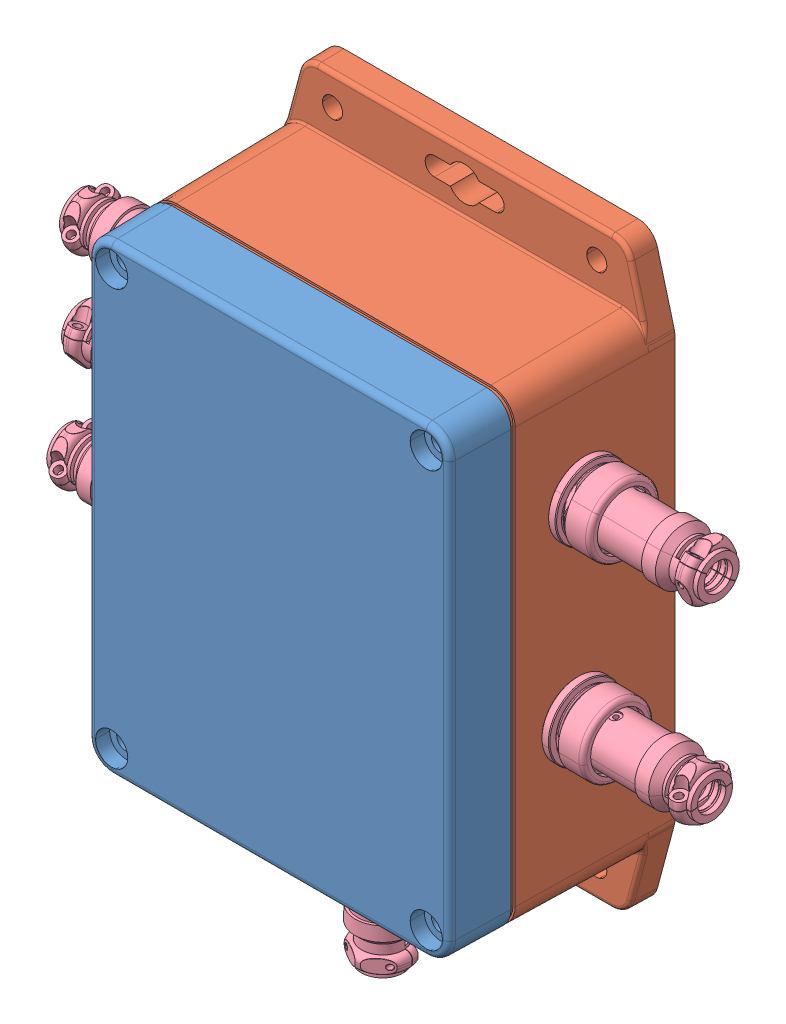
SolidWorks assembly СБ_VelvetADCv.2, configuration Default. Lengths in mm.
Overall size (158.46 164.11 55.04).
10 component instances, 4 part files, 9 mates.
Components (placement in the parent):
- g212mf-g311mf^СБ_VelvetADCv.2-1: g212mf-g311mf^СБ_VelvetADCv.2 [Default] at origin size (91.63 145 55.04) (virtual)
  - G212-COVER^g212mf-g311mf_СБ_VelvetADCv.2-1: G212-COVER^g212mf-g311mf_СБ_VelvetADCv.2 [Default] at (92211.1548 46503.1602 -30.4904) size (90 115 15) (virtual)
  - G212-BASE^g212mf-g311mf_СБ_VelvetADCv.2-1: G212-BASE^g212mf-g311mf_СБ_VelvetADCv.2 [Default] at (92211.1548 46503.1602 -30.4904) size (91.63 145 41.54) (virtual)
- Velvet ADC v2.0^СБ_VelvetADCv.2-1: Velvet ADC v2.0^СБ_VelvetADCv.2 [Default] at (-36.9584 48.4354 -12.2277) x (0 -1 0) z (0 0 1) size (103.38 78.38 22.57) (virtual)
- GX16-4P-1: GX16-4P [Default] at (-76.7536 24.3509 2.2242) x (0.999848 0 -0.017452) z (0.015171 -0.494331 0.869141) size (47.5 21.45 18.91)
- GX16-4P-2: GX16-4P [Default] at (-76.6976 -24.4662 5.4308) x (0.999848 0 -0.017452) z (0.015084 -0.503008 0.86415) size (47.5 21.45 18.91)
- GX16-4P-3: GX16-4P [Default] at (81.2229 24.8878 1.8754) x (-0.999848 0 -0.017452) z (0.014253 -0.577133 -0.816526) size (47.5 21.45 18.91)
- GX16-4P-4: GX16-4P [Default] at (-76.7629 -0.092 1.6932) x (0.999848 0 -0.017452) z (0.016683 0.293639 0.955771) size (47.5 21.45 18.91)
- GX16-4P-5: GX16-4P [Default] at (2.5366 -94.6692 6.5565) x (0 0.999848 -0.017452) z (-0.995263 0.001697 0.097201) size (47.5 21.45 18.91)
- GX16-4P-6: GX16-4P [Default] at (81.1944 -21.6203 3.5074) x (-0.999848 0 -0.017452) z (0.017281 0.139867 -0.99002) size (47.5 21.45 18.91)
Mates (geometry in assembly coordinates):
- Coincident1: coincident anti-aligned: plane of g212mf-g311mf^СБ_VelvetADCv.2-1/G212-BASE^g212mf-g311mf_СБ_VelvetADCv.2-1 through (-31.7684 35.2404 -13.7277) normal (0 0 1); plane of Velvet ADC v2.0.step-1 through (2.2316 -3.2546 -13.7277) normal (0 0 -1)
- Concentric1: concentric aligned: circle of g212mf-g311mf.step-1/G212-BASE.step-1; circle of Velvet ADC v2.0.step-1
- Parallel1: parallel aligned: line of g212mf-g311mf^СБ_VelvetADCv.2-1/G212-BASE^g212mf-g311mf_СБ_VelvetADCv.2-1 through (43.9088 -45.2596 -17.7277) axis (0 1 0); line of Velvet ADC v2.0.step-1 through (41.4216 -46.9296 -12.2277) axis (0 1 0)
- Coincident2: coincident anti-aligned: plane of g212mf-g311mf^СБ_VelvetADCv.2-1/G212-BASE^g212mf-g311mf_СБ_VelvetADCv.2-1 through (-43.4491 -54.6938 -20.7297) normal (-0.999848 0 0.017452); plane of GX16-4P-1 through (-42.9811 32.1743 6.0844) normal (0.999848 0 -0.017452)
- Coincident3: coincident anti-aligned: plane of g212mf-g311mf^СБ_VelvetADCv.2-1/G212-BASE^g212mf-g311mf_СБ_VelvetADCv.2-1 through (-43.4491 -54.6938 -20.7297) normal (-0.999848 0 0.017452); plane of GX16-4P-4 through (-43.1141 8.5113 -1.5373) normal (0.999848 0 -0.017452)
- Coincident4: coincident anti-aligned: plane of g212mf-g311mf^СБ_VelvetADCv.2-1/G212-BASE^g212mf-g311mf_СБ_VelvetADCv.2-1 through (-43.4491 -54.6938 -20.7297) normal (-0.999848 0 0.017452); plane of GX16-4P-2 through (-42.9237 -16.6876 9.369) normal (0.999848 0 -0.017452)
- Coincident5: coincident anti-aligned: plane of g212mf-g311mf^СБ_VelvetADCv.2-1/G212-BASE^g212mf-g311mf_СБ_VelvetADCv.2-1 through (47.9124 48.1746 -20.7297) normal (0.999848 0 0.017452); plane of GX16-4P-3 through (47.6187 32.2377 -3.9062) normal (-0.999848 0 -0.017452)
- Coincident6: coincident anti-aligned: plane of g212mf-g311mf^СБ_VelvetADCv.2-1/G212-BASE^g212mf-g311mf_СБ_VelvetADCv.2-1 through (47.9124 48.1746 -20.7297) normal (0.999848 0 0.017452); plane of GX16-4P-6 through (47.4776 -12.7088 4.1778) normal (-0.999848 0 -0.017452)
- Coincident8: coincident anti-aligned: plane of g212mf-g311mf^СБ_VelvetADCv.2-1/G212-BASE^g212mf-g311mf_СБ_VelvetADCv.2-1 through (2.2316 -60.7596 18.2703) normal (0 -0.999848 0.017452); plane of GX16-4P-5 through (1.6617 -61.1307 -2.9877) normal (0 0.999848 -0.017452)
